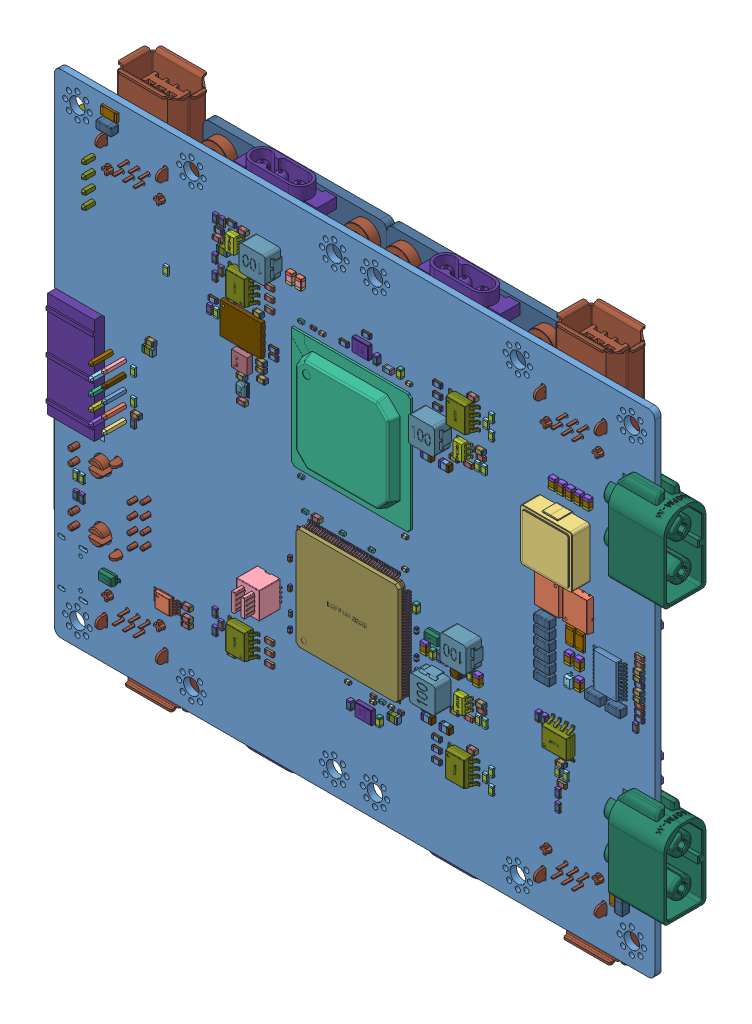
SolidWorks assembly Mother  Board, configuration 默认. Lengths in mm. (continued)
Components (placement in the parent): (continued)
- Mother  Board.step-1: Mother  Board.step [默认] at origin size (122.6 102.08 21) (continued)
  - Free-Models.step-1: Free-Models.step [默认] at origin size (70.87 98.07 8.62) (continued)
    - Driver_Board.step-1: Driver_Board.step [默认] at (49.5407 86.106 -6.2) x (-1 0 0) z (0 0 1) size (35.43 49.03 8.62) (continued)
      - C11-1.step-1: C11-1.step [默认] at origin size (1.6 0.8 0.8)
        - 6547515616.step-1: 6547515616.step [默认] at (27.6859 22.8599 0) x (-1 0 0) z (0 0 1) size (1.6 0.8 0.8)
          - Terminal-22.step-1: Terminal-22.step [默认] at (-0.8 -0.4 0) size (1.6 0.8 0.8)
            - Open_CASCADE_STEP_translator_6.8_47.1.1-85.step-1: Open_CASCADE_STEP_translator_6.8_47.1.1-85.step [默认] at origin size (0.3 0.8 0.8)
            - Open_CASCADE_STEP_translator_6.8_47.1.2-86.step-1: Open_CASCADE_STEP_translator_6.8_47.1.2-86.step [默认] at origin size (0.3 0.8 0.8)
          - Mid_Body-10.step-1: Mid_Body-10.step [默认] at (-0.8 -0.4 0) size (1 0.8 0.8)
            - Open_CASCADE_STEP_translator_6.8_47.2.1-87.step-1: Open_CASCADE_STEP_translator_6.8_47.2.1-87.step [默认] at origin size (1 0.8 0.8)
      - C10-1.step-1: C10-1.step [默认] at origin size (0.8 1.6 0.8)
        - 6547517776.step-1: 6547517776.step [默认] at (-3.1751 37.7191 0) x (0 1 0) z (0 0 1) size (1.6 0.8 0.8)
          - Terminal-24.step-1: Terminal-24.step [默认] at (-0.8 -0.4 0) size (1.6 0.8 0.8)
            - Open_CASCADE_STEP_translator_6.8_47.1.1-104.step-1: Open_CASCADE_STEP_translator_6.8_47.1.1-104.step [默认] at origin size (0.3 0.8 0.8)
            - Open_CASCADE_STEP_translator_6.8_47.1.2-105.step-1: Open_CASCADE_STEP_translator_6.8_47.1.2-105.step [默认] at origin size (0.3 0.8 0.8)
          - Mid_Body-12.step-1: Mid_Body-12.step [默认] at (-0.8 -0.4 0) size (1 0.8 0.8)
            - Open_CASCADE_STEP_translator_6.8_47.2.1-106.step-1: Open_CASCADE_STEP_translator_6.8_47.2.1-106.step [默认] at origin size (1 0.8 0.8)
      - C9-1.step-1: C9-1.step [默认] at origin size (0.8 1.6 0.8)
        - 6547516096.step-1: 6547516096.step [默认] at (-3.1749 22.2249 0) x (0 -1 0) z (0 0 1) size (1.6 0.8 0.8)
          - Terminal-23.step-1: Terminal-23.step [默认] at (-0.8 -0.4 0) size (1.6 0.8 0.8)
            - Open_CASCADE_STEP_translator_6.8_47.1.1-98.step-1: Open_CASCADE_STEP_translator_6.8_47.1.1-98.step [默认] at origin size (0.3 0.8 0.8)
            - Open_CASCADE_STEP_translator_6.8_47.1.2-99.step-1: Open_CASCADE_STEP_translator_6.8_47.1.2-99.step [默认] at origin size (0.3 0.8 0.8)
          - Mid_Body-11.step-1: Mid_Body-11.step [默认] at (-0.8 -0.4 0) size (1 0.8 0.8)
            - Open_CASCADE_STEP_translator_6.8_47.2.1-100.step-1: Open_CASCADE_STEP_translator_6.8_47.2.1-100.step [默认] at origin size (1 0.8 0.8)
      - C8-1.step-1: C8-1.step [默认] at origin size (1.6 0.8 0.8)
        - 6547515616.step-1: 6547515616.step [默认] at (1.1429 16.5099 0) x (-1 0 0) z (0 0 1) size (1.6 0.8 0.8)
          - Terminal-22.step-1: Terminal-22.step [默认] at (-0.8 -0.4 0) size (1.6 0.8 0.8)
            - Open_CASCADE_STEP_translator_6.8_47.1.1-85.step-1: Open_CASCADE_STEP_translator_6.8_47.1.1-85.step [默认] at origin size (0.3 0.8 0.8)
            - Open_CASCADE_STEP_translator_6.8_47.1.2-86.step-1: Open_CASCADE_STEP_translator_6.8_47.1.2-86.step [默认] at origin size (0.3 0.8 0.8)
          - Mid_Body-10.step-1: Mid_Body-10.step [默认] at (-0.8 -0.4 0) size (1 0.8 0.8)
            - Open_CASCADE_STEP_translator_6.8_47.2.1-87.step-1: Open_CASCADE_STEP_translator_6.8_47.2.1-87.step [默认] at origin size (1 0.8 0.8)
      - C7-1.step-1: C7-1.step [默认] at origin size (0.8 1.6 0.8)
        - 6547516096.step-1: 6547516096.step [默认] at (-2.0319 22.2249 0) x (0 -1 0) z (0 0 1) size (1.6 0.8 0.8)
          - Terminal-23.step-1: Terminal-23.step [默认] at (-0.8 -0.4 0) size (1.6 0.8 0.8)
            - Open_CASCADE_STEP_translator_6.8_47.1.1-98.step-1: Open_CASCADE_STEP_translator_6.8_47.1.1-98.step [默认] at origin size (0.3 0.8 0.8)
            - Open_CASCADE_STEP_translator_6.8_47.1.2-99.step-1: Open_CASCADE_STEP_translator_6.8_47.1.2-99.step [默认] at origin size (0.3 0.8 0.8)
          - Mid_Body-11.step-1: Mid_Body-11.step [默认] at (-0.8 -0.4 0) size (1 0.8 0.8)
            - Open_CASCADE_STEP_translator_6.8_47.2.1-100.step-1: Open_CASCADE_STEP_translator_6.8_47.2.1-100.step [默认] at origin size (1 0.8 0.8)
      - C6-1.step-1: C6-1.step [默认] at origin size (0.8 1.6 0.8)
        - 6547517776.step-1: 6547517776.step [默认] at (-2.0321 37.7191 0) x (0 1 0) z (0 0 1) size (1.6 0.8 0.8)
          - Terminal-24.step-1: Terminal-24.step [默认] at (-0.8 -0.4 0) size (1.6 0.8 0.8)
            - Open_CASCADE_STEP_translator_6.8_47.1.1-104.step-1: Open_CASCADE_STEP_translator_6.8_47.1.1-104.step [默认] at origin size (0.3 0.8 0.8)
            - Open_CASCADE_STEP_translator_6.8_47.1.2-105.step-1: Open_CASCADE_STEP_translator_6.8_47.1.2-105.step [默认] at origin size (0.3 0.8 0.8)
          - Mid_Body-12.step-1: Mid_Body-12.step [默认] at (-0.8 -0.4 0) size (1 0.8 0.8)
            - Open_CASCADE_STEP_translator_6.8_47.2.1-106.step-1: Open_CASCADE_STEP_translator_6.8_47.2.1-106.step [默认] at origin size (1 0.8 0.8)
      - C5-1.step-1: C5-1.step [默认] at origin size (1.6 0.8 0.8)
        - 6547515616.step-1: 6547515616.step [默认] at (2.7939 10.6679 0) x (-1 0 0) z (0 0 1) size (1.6 0.8 0.8)
          - Terminal-22.step-1: Terminal-22.step [默认] at (-0.8 -0.4 0) size (1.6 0.8 0.8)
            - Open_CASCADE_STEP_translator_6.8_47.1.1-85.step-1: Open_CASCADE_STEP_translator_6.8_47.1.1-85.step [默认] at origin size (0.3 0.8 0.8)
            - Open_CASCADE_STEP_translator_6.8_47.1.2-86.step-1: Open_CASCADE_STEP_translator_6.8_47.1.2-86.step [默认] at origin size (0.3 0.8 0.8)
          - Mid_Body-10.step-1: Mid_Body-10.step [默认] at (-0.8 -0.4 0) size (1 0.8 0.8)
            - Open_CASCADE_STEP_translator_6.8_47.2.1-87.step-1: Open_CASCADE_STEP_translator_6.8_47.2.1-87.step [默认] at origin size (1 0.8 0.8)
      - C4-1.step-1: C4-1.step [默认] at origin size (1.6 0.8 0.8)
        - 6547515616.step-1: 6547515616.step [默认] at (-0.1271 22.8599 0) x (-1 0 0) z (0 0 1) size (1.6 0.8 0.8)
          - Terminal-22.step-1: Terminal-22.step [默认] at (-0.8 -0.4 0) size (1.6 0.8 0.8)
            - Open_CASCADE_STEP_translator_6.8_47.1.1-85.step-1: Open_CASCADE_STEP_translator_6.8_47.1.1-85.step [默认] at origin size (0.3 0.8 0.8)
            - Open_CASCADE_STEP_translator_6.8_47.1.2-86.step-1: Open_CASCADE_STEP_translator_6.8_47.1.2-86.step [默认] at origin size (0.3 0.8 0.8)
          - Mid_Body-10.step-1: Mid_Body-10.step [默认] at (-0.8 -0.4 0) size (1 0.8 0.8)
            - Open_CASCADE_STEP_translator_6.8_47.2.1-87.step-1: Open_CASCADE_STEP_translator_6.8_47.2.1-87.step [默认] at origin size (1 0.8 0.8)
      - C3-1.step-1: C3-1.step [默认] at origin size (2.01 1.25 0.94)
        - 6547513136.step-1: 6547513136.step [默认] at (6.6263 23.4725 0) x (-1 0 0) z (0 0 1) size (2.01 1.25 0.94)
          - Fillet1-95.step-1: Fillet1-95.step [默认] at origin size (0.5 1.25 0.94)
          - Fillet2-96.step-1: Fillet2-96.step [默认] at origin size (0.5 1.25 0.94)
          - body2-97.step-1: body2-97.step [默认] at origin size (1.01 1.22 0.92)
      - C2-1.step-1: C2-1.step [默认] at origin size (0.8 1.6 0.8)
        - 6547516096.step-1: 6547516096.step [默认] at (3.7055 24.7425 0) x (0 -1 0) z (0 0 1) size (1.6 0.8 0.8)
          - Terminal-23.step-1: Terminal-23.step [默认] at (-0.8 -0.4 0) size (1.6 0.8 0.8)
            - Open_CASCADE_STEP_translator_6.8_47.1.1-98.step-1: Open_CASCADE_STEP_translator_6.8_47.1.1-98.step [默认] at origin size (0.3 0.8 0.8)
            - Open_CASCADE_STEP_translator_6.8_47.1.2-99.step-1: Open_CASCADE_STEP_translator_6.8_47.1.2-99.step [默认] at origin size (0.3 0.8 0.8)
          - Mid_Body-11.step-1: Mid_Body-11.step [默认] at (-0.8 -0.4 0) size (1 0.8 0.8)
            - Open_CASCADE_STEP_translator_6.8_47.2.1-100.step-1: Open_CASCADE_STEP_translator_6.8_47.2.1-100.step [默认] at origin size (1 0.8 0.8)
      - C1.step-1: C1.step [默认] at origin size (1.25 2.01 0.94)
        - 6547514896.step-1: 6547514896.step [默认] at (9.2933 31.0126 0) x (0 1 0) z (0 0 1) size (2.01 1.25 0.94)
          - Fillet1-101.step-1: Fillet1-101.step [默认] at origin size (0.5 1.25 0.94)
          - Fillet2-102.step-1: Fillet2-102.step [默认] at origin size (0.5 1.25 0.94)
          - body2-103.step-1: body2-103.step [默认] at origin size (1.01 1.22 0.92)
    - Driver_Board.step-2: Driver_Board.step [默认] at (84.963 86.106 -6.2) x (-1 0 0) z (0 0 1) size (35.43 49.03 8.62)
      - Board-1.step-1: Board-1.step [默认] at origin size (35.43 46.99 1.62)
        - Open_CASCADE_STEP_translator_6.8_2.1.1.step-1: Open_CASCADE_STEP_translator_6.8_2.1.1.step [默认] at (0 0 -1.6164) size (35.43 46.99 1.62)
      - R25-1.step-1: R25-1.step [默认] at origin size (0.8 1.6 0.45)
        - 6547515376.step-1: 6547515376.step [默认] at (20.6304 35.5601 0) x (0 1 0) z (0 0 1) size (1.6 0.8 0.45)
          - Terminal-19.step-1: Terminal-19.step [默认] at (-0.8 -0.4 0) size (0.3 0.8 0.45)
            - Open_CASCADE_STEP_translator_6.8_21.2.1-76.step-1: Open_CASCADE_STEP_translator_6.8_21.2.1-76.step [默认] at origin size (0.3 0.8 0.45)
          - Terminal-19.step-2: Terminal-19.step [默认] at (0.8 0.4 0) x (-1 0 0) z (0 0 1) size (0.3 0.8 0.45)
            - Open_CASCADE_STEP_translator_6.8_21.2.1-76.step-1: Open_CASCADE_STEP_translator_6.8_21.2.1-76.step [默认] at origin size (0.3 0.8 0.45)
          - Mid_Body-77.step-1: Mid_Body-77.step [默认] at (-0.8 -0.4 0) size (1.51 0.8 0.36)
          - Mark-78.step-1: Mark-78.step [默认] at (-0.5 -0.4 0.405) size (1 0.8 0.05)
      - R24-1.step-1: R24-1.step [默认] at origin size (1.6 0.8 0.45)
        - 6547516336.step-1: 6547516336.step [默认] at (12.6999 34.9249 0) x (-1 0 0) z (0 0 1) size (1.6 0.8 0.45)
          - Terminal-20.step-1: Terminal-20.step [默认] at (-0.8 -0.4 0) size (0.3 0.8 0.45)
            - Open_CASCADE_STEP_translator_6.8_21.2.1-79.step-1: Open_CASCADE_STEP_translator_6.8_21.2.1-79.step [默认] at origin size (0.3 0.8 0.45)
          - Terminal-20.step-2: Terminal-20.step [默认] at (0.8 0.4 0) x (-1 0 0) z (0 0 1) size (0.3 0.8 0.45)
            - Open_CASCADE_STEP_translator_6.8_21.2.1-79.step-1: Open_CASCADE_STEP_translator_6.8_21.2.1-79.step [默认] at origin size (0.3 0.8 0.45)
          - Mid_Body-80.step-1: Mid_Body-80.step [默认] at (-0.8 -0.4 0) size (1.51 0.8 0.36)
          - Mark-81.step-1: Mark-81.step [默认] at (-0.5 -0.4 0.405) size (1 0.8 0.05)
      - R23-1.step-1: R23-1.step [默认] at origin size (1.6 0.8 0.45)
        - 6547516336.step-1: 6547516336.step [默认] at (5.5879 33.6549 0) x (-1 0 0) z (0 0 1) size (1.6 0.8 0.45)
          - Terminal-20.step-1: Terminal-20.step [默认] at (-0.8 -0.4 0) size (0.3 0.8 0.45)
            - Open_CASCADE_STEP_translator_6.8_21.2.1-79.step-1: Open_CASCADE_STEP_translator_6.8_21.2.1-79.step [默认] at origin size (0.3 0.8 0.45)
          - Terminal-20.step-2: Terminal-20.step [默认] at (0.8 0.4 0) x (-1 0 0) z (0 0 1) size (0.3 0.8 0.45)
            - Open_CASCADE_STEP_translator_6.8_21.2.1-79.step-1: Open_CASCADE_STEP_translator_6.8_21.2.1-79.step [默认] at origin size (0.3 0.8 0.45)
          - Mid_Body-80.step-1: Mid_Body-80.step [默认] at (-0.8 -0.4 0) size (1.51 0.8 0.36)
          - Mark-81.step-1: Mark-81.step [默认] at (-0.5 -0.4 0.405) size (1 0.8 0.05)
      - JP1.step-1: JP1.step [默认] at origin size (16.01 14.49 6.96)
        - User_Library-MR30PW-M.step-1: User_Library-MR30PW-M.step [默认] at (13.7158 -5.9802 2.75) x (1 0 0) z (0 0 1) size (16.01 14.49 6.96)
      - R18-1.step-1: R18-1.step [默认] at origin size (0.8 1.6 0.45)
        - 6547515376.step-1: 6547515376.step [默认] at (22.9869 34.4171 0) x (0 1 0) z (0 0 1) size (1.6 0.8 0.45)
          - Terminal-19.step-1: Terminal-19.step [默认] at (-0.8 -0.4 0) size (0.3 0.8 0.45)
            - Open_CASCADE_STEP_translator_6.8_21.2.1-76.step-1: Open_CASCADE_STEP_translator_6.8_21.2.1-76.step [默认] at origin size (0.3 0.8 0.45)
          - Terminal-19.step-2: Terminal-19.step [默认] at (0.8 0.4 0) x (-1 0 0) z (0 0 1) size (0.3 0.8 0.45)
            - Open_CASCADE_STEP_translator_6.8_21.2.1-76.step-1: Open_CASCADE_STEP_translator_6.8_21.2.1-76.step [默认] at origin size (0.3 0.8 0.45)
          - Mid_Body-77.step-1: Mid_Body-77.step [默认] at (-0.8 -0.4 0) size (1.51 0.8 0.36)
          - Mark-78.step-1: Mark-78.step [默认] at (-0.5 -0.4 0.405) size (1 0.8 0.05)
      - R17-1.step-1: R17-1.step [默认] at origin size (0.8 1.6 0.45)
        - 6547515376.step-1: 6547515376.step [默认] at (21.8663 34.3947 0) x (0 1 0) z (0 0 1) size (1.6 0.8 0.45)
          - Terminal-19.step-1: Terminal-19.step [默认] at (-0.8 -0.4 0) size (0.3 0.8 0.45)
            - Open_CASCADE_STEP_translator_6.8_21.2.1-76.step-1: Open_CASCADE_STEP_translator_6.8_21.2.1-76.step [默认] at origin size (0.3 0.8 0.45)
          - Terminal-19.step-2: Terminal-19.step [默认] at (0.8 0.4 0) x (-1 0 0) z (0 0 1) size (0.3 0.8 0.45)
            - Open_CASCADE_STEP_translator_6.8_21.2.1-76.step-1: Open_CASCADE_STEP_translator_6.8_21.2.1-76.step [默认] at origin size (0.3 0.8 0.45)
          - Mid_Body-77.step-1: Mid_Body-77.step [默认] at (-0.8 -0.4 0) size (1.51 0.8 0.36)
          - Mark-78.step-1: Mark-78.step [默认] at (-0.5 -0.4 0.405) size (1 0.8 0.05)
      - R16-1.step-1: R16-1.step [默认] at origin size (1.6 0.8 0.45)
        - 6547506496.step-1: 6547506496.step [默认] at (16.6371 33.6551 0) x (1 0 0) z (0 0 1) size (1.6 0.8 0.45)
          - Terminal-21.step-1: Terminal-21.step [默认] at (-0.8 -0.4 0) size (0.3 0.8 0.45)
            - Open_CASCADE_STEP_translator_6.8_21.2.1-82.step-1: Open_CASCADE_STEP_translator_6.8_21.2.1-82.step [默认] at origin size (0.3 0.8 0.45)
          - Terminal-21.step-2: Terminal-21.step [默认] at (0.8 0.4 0) x (-1 0 0) z (0 0 1) size (0.3 0.8 0.45)
            - Open_CASCADE_STEP_translator_6.8_21.2.1-82.step-1: Open_CASCADE_STEP_translator_6.8_21.2.1-82.step [默认] at origin size (0.3 0.8 0.45)
          - Mid_Body-83.step-1: Mid_Body-83.step [默认] at (-0.8 -0.4 0) size (1.51 0.8 0.36)
          - Mark-84.step-1: Mark-84.step [默认] at (-0.5 -0.4 0.405) size (1 0.8 0.05)
      - R15-1.step-1: R15-1.step [默认] at origin size (0.8 1.6 0.45)
        - 6547515376.step-1: 6547515376.step [默认] at (14.7319 34.2901 0) x (0 1 0) z (0 0 1) size (1.6 0.8 0.45)
          - Terminal-19.step-1: Terminal-19.step [默认] at (-0.8 -0.4 0) size (0.3 0.8 0.45)
            - Open_CASCADE_STEP_translator_6.8_21.2.1-76.step-1: Open_CASCADE_STEP_translator_6.8_21.2.1-76.step [默认] at origin size (0.3 0.8 0.45)
          - Terminal-19.step-2: Terminal-19.step [默认] at (0.8 0.4 0) x (-1 0 0) z (0 0 1) size (0.3 0.8 0.45)
            - Open_CASCADE_STEP_translator_6.8_21.2.1-76.step-1: Open_CASCADE_STEP_translator_6.8_21.2.1-76.step [默认] at origin size (0.3 0.8 0.45)
          - Mid_Body-77.step-1: Mid_Body-77.step [默认] at (-0.8 -0.4 0) size (1.51 0.8 0.36)
          - Mark-78.step-1: Mark-78.step [默认] at (-0.5 -0.4 0.405) size (1 0.8 0.05)
      - R13-1.step-1: R13-1.step [默认] at origin size (1.6 0.8 0.45)
        - 6547506496.step-1: 6547506496.step [默认] at (9.5251 33.6551 0) x (1 0 0) z (0 0 1) size (1.6 0.8 0.45)
          - Terminal-21.step-1: Terminal-21.step [默认] at (-0.8 -0.4 0) size (0.3 0.8 0.45)
            - Open_CASCADE_STEP_translator_6.8_21.2.1-82.step-1: Open_CASCADE_STEP_translator_6.8_21.2.1-82.step [默认] at origin size (0.3 0.8 0.45)
          - Terminal-21.step-2: Terminal-21.step [默认] at (0.8 0.4 0) x (-1 0 0) z (0 0 1) size (0.3 0.8 0.45)
            - Open_CASCADE_STEP_translator_6.8_21.2.1-82.step-1: Open_CASCADE_STEP_translator_6.8_21.2.1-82.step [默认] at origin size (0.3 0.8 0.45)
          - Mid_Body-83.step-1: Mid_Body-83.step [默认] at (-0.8 -0.4 0) size (1.51 0.8 0.36)
          - Mark-84.step-1: Mark-84.step [默认] at (-0.5 -0.4 0.405) size (1 0.8 0.05)
      - R11-1.step-1: R11-1.step [默认] at origin size (0.8 1.6 0.45)
        - 6547515376.step-1: 6547515376.step [默认] at (7.6423 34.2901 0) x (0 1 0) z (0 0 1) size (1.6 0.8 0.45)
          - Terminal-19.step-1: Terminal-19.step [默认] at (-0.8 -0.4 0) size (0.3 0.8 0.45)
            - Open_CASCADE_STEP_translator_6.8_21.2.1-76.step-1: Open_CASCADE_STEP_translator_6.8_21.2.1-76.step [默认] at origin size (0.3 0.8 0.45)
          - Terminal-19.step-2: Terminal-19.step [默认] at (0.8 0.4 0) x (-1 0 0) z (0 0 1) size (0.3 0.8 0.45)
            - Open_CASCADE_STEP_translator_6.8_21.2.1-76.step-1: Open_CASCADE_STEP_translator_6.8_21.2.1-76.step [默认] at origin size (0.3 0.8 0.45)
          - Mid_Body-77.step-1: Mid_Body-77.step [默认] at (-0.8 -0.4 0) size (1.51 0.8 0.36)
          - Mark-78.step-1: Mark-78.step [默认] at (-0.5 -0.4 0.405) size (1 0.8 0.05)
      - C23-1.step-1: C23-1.step [默认] at origin size (1.6 0.8 0.8)
        - 6547515616.step-1: 6547515616.step [默认] at (19.8684 33.6676 0) x (-1 0 0) z (0 0 1) size (1.6 0.8 0.8)
          - Terminal-22.step-1: Terminal-22.step [默认] at (-0.8 -0.4 0) size (1.6 0.8 0.8)
            - Open_CASCADE_STEP_translator_6.8_47.1.1-85.step-1: Open_CASCADE_STEP_translator_6.8_47.1.1-85.step [默认] at origin size (0.3 0.8 0.8)
            - Open_CASCADE_STEP_translator_6.8_47.1.2-86.step-1: Open_CASCADE_STEP_translator_6.8_47.1.2-86.step [默认] at origin size (0.3 0.8 0.8)
          - Mid_Body-10.step-1: Mid_Body-10.step [默认] at (-0.8 -0.4 0) size (1 0.8 0.8)
            - Open_CASCADE_STEP_translator_6.8_47.2.1-87.step-1: Open_CASCADE_STEP_translator_6.8_47.2.1-87.step [默认] at origin size (1 0.8 0.8)
      - C22-1.step-1: C22-1.step [默认] at origin size (1.6 0.8 0.8)
        - 6547515616.step-1: 6547515616.step [默认] at (12.6999 33.6549 0) x (-1 0 0) z (0 0 1) size (1.6 0.8 0.8)
          - Terminal-22.step-1: Terminal-22.step [默认] at (-0.8 -0.4 0) size (1.6 0.8 0.8)
            - Open_CASCADE_STEP_translator_6.8_47.1.1-85.step-1: Open_CASCADE_STEP_translator_6.8_47.1.1-85.step [默认] at origin size (0.3 0.8 0.8)
            - Open_CASCADE_STEP_translator_6.8_47.1.2-86.step-1: Open_CASCADE_STEP_translator_6.8_47.1.2-86.step [默认] at origin size (0.3 0.8 0.8)
          - Mid_Body-10.step-1: Mid_Body-10.step [默认] at (-0.8 -0.4 0) size (1 0.8 0.8)
            - Open_CASCADE_STEP_translator_6.8_47.2.1-87.step-1: Open_CASCADE_STEP_translator_6.8_47.2.1-87.step [默认] at origin size (1 0.8 0.8)
      - C21-1.step-1: C21-1.step [默认] at origin size (1.6 0.8 0.8)
        - 6547515616.step-1: 6547515616.step [默认] at (5.6103 34.9025 0) x (-1 0 0) z (0 0 1) size (1.6 0.8 0.8)
          - Terminal-22.step-1: Terminal-22.step [默认] at (-0.8 -0.4 0) size (1.6 0.8 0.8)
            - Open_CASCADE_STEP_translator_6.8_47.1.1-85.step-1: Open_CASCADE_STEP_translator_6.8_47.1.1-85.step [默认] at origin size (0.3 0.8 0.8)
            - Open_CASCADE_STEP_translator_6.8_47.1.2-86.step-1: Open_CASCADE_STEP_translator_6.8_47.1.2-86.step [默认] at origin size (0.3 0.8 0.8)
          - Mid_Body-10.step-1: Mid_Body-10.step [默认] at (-0.8 -0.4 0) size (1 0.8 0.8)
            - Open_CASCADE_STEP_translator_6.8_47.2.1-87.step-1: Open_CASCADE_STEP_translator_6.8_47.2.1-87.step [默认] at origin size (1 0.8 0.8)
      - U5-1.step-1: U5-1.step [默认] at origin size (5.9 11.5 2.7)
        - SO8_W.step-1: SO8_W.step [默认] at (27.6859 29.9721 0.381) x (0 1 0) z (0 0 1) size (11.5 5.9 2.7)
      - U4-1.step-1: U4-1.step [默认] at origin size (5.9 11.5 2.7)
        - SO8_W.step-1: SO8_W.step [默认] at (-0.1271 29.9721 0.381) x (0 1 0) z (0 0 1) size (11.5 5.9 2.7)
      - U3-1.step-1: U3-1.step [默认] at origin size (5 6.01 1.9)
        - SOP8-1.step-1: SOP8-1.step [默认] at (19.9615 29.5285 0) x (0 -1 0) z (0 0 1) size (6.01 5 1.9)
          - LOGO_-88.step-1: LOGO_-88.step [默认] at (0.0116 0 0.095) x (0 -1 0) z (0 0 -1) size (1.5 1.73 0.01)
          - SOP8-89.step-1: SOP8-89.step [默认] at origin size (6.01 5 1.9)
      - U2-1.step-1: U2-1.step [默认] at origin size (5 6.01 1.9)
        - SOP8-1.step-1: SOP8-1.step [默认] at (12.8495 29.5285 0) x (0 -1 0) z (0 0 1) size (6.01 5 1.9)
          - LOGO_-88.step-1: LOGO_-88.step [默认] at (0.0116 0 0.095) x (0 -1 0) z (0 0 -1) size (1.5 1.73 0.01)
          - SOP8-89.step-1: SOP8-89.step [默认] at origin size (6.01 5 1.9)
      - U1.step-1: U1.step [默认] at origin size (5 6.01 1.9)
        - SOP8-1.step-1: SOP8-1.step [默认] at (5.7375 29.5285 0) x (0 -1 0) z (0 0 1) size (6.01 5 1.9)
          - LOGO_-88.step-1: LOGO_-88.step [默认] at (0.0116 0 0.095) x (0 -1 0) z (0 0 -1) size (1.5 1.73 0.01)
          - SOP8-89.step-1: SOP8-89.step [默认] at origin size (6.01 5 1.9)
      - RS2-1.step-1: RS2-1.step [默认] at origin size (3.1 1.55 0.47)
        - User_Library-R1206-90.step-1: User_Library-R1206-90.step [默认] at (23.7489 17.5261 -1.6164) x (-1 0 0) z (0 0 -1) size (3.1 1.55 0.47)
      - RS1-1.step-1: RS1-1.step [默认] at origin size (3.1 1.55 0.47)
        - User_Library-R1206-90.step-1: User_Library-R1206-90.step [默认] at (-0.1271 18.1611 -1.6164) x (-1 0 0) z (0 0 -1) size (3.1 1.55 0.47)
      - R22-1.step-1: R22-1.step [默认] at origin size (1.6 0.8 0.45)
        - 6547506496.step-1: 6547506496.step [默认] at (22.9871 17.7801 0) x (1 0 0) z (0 0 1) size (1.6 0.8 0.45)
          - Terminal-21.step-1: Terminal-21.step [默认] at (-0.8 -0.4 0) size (0.3 0.8 0.45)
            - Open_CASCADE_STEP_translator_6.8_21.2.1-82.step-1: Open_CASCADE_STEP_translator_6.8_21.2.1-82.step [默认] at origin size (0.3 0.8 0.45)
          - Terminal-21.step-2: Terminal-21.step [默认] at (0.8 0.4 0) x (-1 0 0) z (0 0 1) size (0.3 0.8 0.45)
            - Open_CASCADE_STEP_translator_6.8_21.2.1-82.step-1: Open_CASCADE_STEP_translator_6.8_21.2.1-82.step [默认] at origin size (0.3 0.8 0.45)
          - Mid_Body-83.step-1: Mid_Body-83.step [默认] at (-0.8 -0.4 0) size (1.51 0.8 0.36)
          - Mark-84.step-1: Mark-84.step [默认] at (-0.5 -0.4 0.405) size (1 0.8 0.05)
      - R21-1.step-1: R21-1.step [默认] at origin size (1.6 0.8 0.45)
        - 6547516336.step-1: 6547516336.step [默认] at (22.9869 18.9229 0) x (-1 0 0) z (0 0 1) size (1.6 0.8 0.45)
          - Terminal-20.step-1: Terminal-20.step [默认] at (-0.8 -0.4 0) size (0.3 0.8 0.45)
            - Open_CASCADE_STEP_translator_6.8_21.2.1-79.step-1: Open_CASCADE_STEP_translator_6.8_21.2.1-79.step [默认] at origin size (0.3 0.8 0.45)
          - Terminal-20.step-2: Terminal-20.step [默认] at (0.8 0.4 0) x (-1 0 0) z (0 0 1) size (0.3 0.8 0.45)
            - Open_CASCADE_STEP_translator_6.8_21.2.1-79.step-1: Open_CASCADE_STEP_translator_6.8_21.2.1-79.step [默认] at origin size (0.3 0.8 0.45)
          - Mid_Body-80.step-1: Mid_Body-80.step [默认] at (-0.8 -0.4 0) size (1.51 0.8 0.36)
          - Mark-81.step-1: Mark-81.step [默认] at (-0.5 -0.4 0.405) size (1 0.8 0.05)
      - R20-1.step-1: R20-1.step [默认] at origin size (1.6 0.8 0.45)
        - 6547506496.step-1: 6547506496.step [默认] at (24.6381 11.8111 0) x (1 0 0) z (0 0 1) size (1.6 0.8 0.45)
          - Terminal-21.step-1: Terminal-21.step [默认] at (-0.8 -0.4 0) size (0.3 0.8 0.45)
            - Open_CASCADE_STEP_translator_6.8_21.2.1-82.step-1: Open_CASCADE_STEP_translator_6.8_21.2.1-82.step [默认] at origin size (0.3 0.8 0.45)
          - Terminal-21.step-2: Terminal-21.step [默认] at (0.8 0.4 0) x (-1 0 0) z (0 0 1) size (0.3 0.8 0.45)
            - Open_CASCADE_STEP_translator_6.8_21.2.1-82.step-1: Open_CASCADE_STEP_translator_6.8_21.2.1-82.step [默认] at origin size (0.3 0.8 0.45)
          - Mid_Body-83.step-1: Mid_Body-83.step [默认] at (-0.8 -0.4 0) size (1.51 0.8 0.36)
          - Mark-84.step-1: Mark-84.step [默认] at (-0.5 -0.4 0.405) size (1 0.8 0.05)
      - R19-1.step-1: R19-1.step [默认] at origin size (0.8 1.6 0.45)
        - 6547515376.step-1: 6547515376.step [默认] at (25.3999 13.5891 0) x (0 1 0) z (0 0 1) size (1.6 0.8 0.45)
          - Terminal-19.step-1: Terminal-19.step [默认] at (-0.8 -0.4 0) size (0.3 0.8 0.45)
            - Open_CASCADE_STEP_translator_6.8_21.2.1-76.step-1: Open_CASCADE_STEP_translator_6.8_21.2.1-76.step [默认] at origin size (0.3 0.8 0.45)
          - Terminal-19.step-2: Terminal-19.step [默认] at (0.8 0.4 0) x (-1 0 0) z (0 0 1) size (0.3 0.8 0.45)
            - Open_CASCADE_STEP_translator_6.8_21.2.1-76.step-1: Open_CASCADE_STEP_translator_6.8_21.2.1-76.step [默认] at origin size (0.3 0.8 0.45)
          - Mid_Body-77.step-1: Mid_Body-77.step [默认] at (-0.8 -0.4 0) size (1.51 0.8 0.36)
          - Mark-78.step-1: Mark-78.step [默认] at (-0.5 -0.4 0.405) size (1 0.8 0.05)
      - R14-1.step-1: R14-1.step [默认] at origin size (1.6 0.8 0.45)
        - 6547506496.step-1: 6547506496.step [默认] at (12.0651 20.0661 0) x (1 0 0) z (0 0 1) size (1.6 0.8 0.45)
          - Terminal-21.step-1: Terminal-21.step [默认] at (-0.8 -0.4 0) size (0.3 0.8 0.45)
            - Open_CASCADE_STEP_translator_6.8_21.2.1-82.step-1: Open_CASCADE_STEP_translator_6.8_21.2.1-82.step [默认] at origin size (0.3 0.8 0.45)
          - Terminal-21.step-2: Terminal-21.step [默认] at (0.8 0.4 0) x (-1 0 0) z (0 0 1) size (0.3 0.8 0.45)
            - Open_CASCADE_STEP_translator_6.8_21.2.1-82.step-1: Open_CASCADE_STEP_translator_6.8_21.2.1-82.step [默认] at origin size (0.3 0.8 0.45)
          - Mid_Body-83.step-1: Mid_Body-83.step [默认] at (-0.8 -0.4 0) size (1.51 0.8 0.36)
          - Mark-84.step-1: Mark-84.step [默认] at (-0.5 -0.4 0.405) size (1 0.8 0.05)
      - R12-1.step-1: R12-1.step [默认] at origin size (1.6 0.8 0.45)
        - 6547516336.step-1: 6547516336.step [默认] at (12.0649 21.2089 0) x (-1 0 0) z (0 0 1) size (1.6 0.8 0.45)
          - Terminal-20.step-1: Terminal-20.step [默认] at (-0.8 -0.4 0) size (0.3 0.8 0.45)
            - Open_CASCADE_STEP_translator_6.8_21.2.1-79.step-1: Open_CASCADE_STEP_translator_6.8_21.2.1-79.step [默认] at origin size (0.3 0.8 0.45)
          - Terminal-20.step-2: Terminal-20.step [默认] at (0.8 0.4 0) x (-1 0 0) z (0 0 1) size (0.3 0.8 0.45)
            - Open_CASCADE_STEP_translator_6.8_21.2.1-79.step-1: Open_CASCADE_STEP_translator_6.8_21.2.1-79.step [默认] at origin size (0.3 0.8 0.45)
          - Mid_Body-80.step-1: Mid_Body-80.step [默认] at (-0.8 -0.4 0) size (1.51 0.8 0.36)
          - Mark-81.step-1: Mark-81.step [默认] at (-0.5 -0.4 0.405) size (1 0.8 0.05)
      - R10-1.step-1: R10-1.step [默认] at origin size (1.6 0.8 0.45)
        - 6547506496.step-1: 6547506496.step [默认] at (13.7161 14.0971 0) x (1 0 0) z (0 0 1) size (1.6 0.8 0.45)
          - Terminal-21.step-1: Terminal-21.step [默认] at (-0.8 -0.4 0) size (0.3 0.8 0.45)
            - Open_CASCADE_STEP_translator_6.8_21.2.1-82.step-1: Open_CASCADE_STEP_translator_6.8_21.2.1-82.step [默认] at origin size (0.3 0.8 0.45)
          - Terminal-21.step-2: Terminal-21.step [默认] at (0.8 0.4 0) x (-1 0 0) z (0 0 1) size (0.3 0.8 0.45)
            - Open_CASCADE_STEP_translator_6.8_21.2.1-82.step-1: Open_CASCADE_STEP_translator_6.8_21.2.1-82.step [默认] at origin size (0.3 0.8 0.45)
          - Mid_Body-83.step-1: Mid_Body-83.step [默认] at (-0.8 -0.4 0) size (1.51 0.8 0.36)
          - Mark-84.step-1: Mark-84.step [默认] at (-0.5 -0.4 0.405) size (1 0.8 0.05)
      - R9-1.step-1: R9-1.step [默认] at origin size (0.8 1.6 0.45)
        - 6547515376.step-1: 6547515376.step [默认] at (14.4779 15.8751 0) x (0 1 0) z (0 0 1) size (1.6 0.8 0.45)
          - Terminal-19.step-1: Terminal-19.step [默认] at (-0.8 -0.4 0) size (0.3 0.8 0.45)
            - Open_CASCADE_STEP_translator_6.8_21.2.1-76.step-1: Open_CASCADE_STEP_translator_6.8_21.2.1-76.step [默认] at origin size (0.3 0.8 0.45)
          - Terminal-19.step-2: Terminal-19.step [默认] at (0.8 0.4 0) x (-1 0 0) z (0 0 1) size (0.3 0.8 0.45)
            - Open_CASCADE_STEP_translator_6.8_21.2.1-76.step-1: Open_CASCADE_STEP_translator_6.8_21.2.1-76.step [默认] at origin size (0.3 0.8 0.45)
          - Mid_Body-77.step-1: Mid_Body-77.step [默认] at (-0.8 -0.4 0) size (1.51 0.8 0.36)
          - Mark-78.step-1: Mark-78.step [默认] at (-0.5 -0.4 0.405) size (1 0.8 0.05)
      - R8-1.step-1: R8-1.step [默认] at origin size (0.8 1.6 0.45)
        - 6547515376.step-1: 6547515376.step [默认] at (28.3209 21.0821 0) x (0 1 0) z (0 0 1) size (1.6 0.8 0.45)
          - Terminal-19.step-1: Terminal-19.step [默认] at (-0.8 -0.4 0) size (0.3 0.8 0.45)
            - Open_CASCADE_STEP_translator_6.8_21.2.1-76.step-1: Open_CASCADE_STEP_translator_6.8_21.2.1-76.step [默认] at origin size (0.3 0.8 0.45)
          - Terminal-19.step-2: Terminal-19.step [默认] at (0.8 0.4 0) x (-1 0 0) z (0 0 1) size (0.3 0.8 0.45)
            - Open_CASCADE_STEP_translator_6.8_21.2.1-76.step-1: Open_CASCADE_STEP_translator_6.8_21.2.1-76.step [默认] at origin size (0.3 0.8 0.45)
          - Mid_Body-77.step-1: Mid_Body-77.step [默认] at (-0.8 -0.4 0) size (1.51 0.8 0.36)
          - Mark-78.step-1: Mark-78.step [默认] at (-0.5 -0.4 0.405) size (1 0.8 0.05)
      - R7-1.step-1: R7-1.step [默认] at origin size (0.8 1.6 0.45)
        - 6547515376.step-1: 6547515376.step [默认] at (27.0509 21.0821 0) x (0 1 0) z (0 0 1) size (1.6 0.8 0.45)
          - Terminal-19.step-1: Terminal-19.step [默认] at (-0.8 -0.4 0) size (0.3 0.8 0.45)
            - Open_CASCADE_STEP_translator_6.8_21.2.1-76.step-1: Open_CASCADE_STEP_translator_6.8_21.2.1-76.step [默认] at origin size (0.3 0.8 0.45)
          - Terminal-19.step-2: Terminal-19.step [默认] at (0.8 0.4 0) x (-1 0 0) z (0 0 1) size (0.3 0.8 0.45)
            - Open_CASCADE_STEP_translator_6.8_21.2.1-76.step-1: Open_CASCADE_STEP_translator_6.8_21.2.1-76.step [默认] at origin size (0.3 0.8 0.45)
          - Mid_Body-77.step-1: Mid_Body-77.step [默认] at (-0.8 -0.4 0) size (1.51 0.8 0.36)
          - Mark-78.step-1: Mark-78.step [默认] at (-0.5 -0.4 0.405) size (1 0.8 0.05)
      - R6.step-1: R6.step [默认] at origin size (1.6 0.8 0.45)
        - 6547506496.step-1: 6547506496.step [默认] at (1.1431 17.6531 0) x (1 0 0) z (0 0 1) size (1.6 0.8 0.45)
          - Terminal-21.step-1: Terminal-21.step [默认] at (-0.8 -0.4 0) size (0.3 0.8 0.45)
            - Open_CASCADE_STEP_translator_6.8_21.2.1-82.step-1: Open_CASCADE_STEP_translator_6.8_21.2.1-82.step [默认] at origin size (0.3 0.8 0.45)
          - Terminal-21.step-2: Terminal-21.step [默认] at (0.8 0.4 0) x (-1 0 0) z (0 0 1) size (0.3 0.8 0.45)
            - Open_CASCADE_STEP_translator_6.8_21.2.1-82.step-1: Open_CASCADE_STEP_translator_6.8_21.2.1-82.step [默认] at origin size (0.3 0.8 0.45)
          - Mid_Body-83.step-1: Mid_Body-83.step [默认] at (-0.8 -0.4 0) size (1.51 0.8 0.36)
          - Mark-84.step-1: Mark-84.step [默认] at (-0.5 -0.4 0.405) size (1 0.8 0.05)
      - R5.step-1: R5.step [默认] at origin size (0.8 1.6 0.45)
        - 6547515376.step-1: 6547515376.step [默认] at (1.7779 21.0821 0) x (0 1 0) z (0 0 1) size (1.6 0.8 0.45)
          - Terminal-19.step-1: Terminal-19.step [默认] at (-0.8 -0.4 0) size (0.3 0.8 0.45)
            - Open_CASCADE_STEP_translator_6.8_21.2.1-76.step-1: Open_CASCADE_STEP_translator_6.8_21.2.1-76.step [默认] at origin size (0.3 0.8 0.45)
          - Terminal-19.step-2: Terminal-19.step [默认] at (0.8 0.4 0) x (-1 0 0) z (0 0 1) size (0.3 0.8 0.45)
            - Open_CASCADE_STEP_translator_6.8_21.2.1-76.step-1: Open_CASCADE_STEP_translator_6.8_21.2.1-76.step [默认] at origin size (0.3 0.8 0.45)
          - Mid_Body-77.step-1: Mid_Body-77.step [默认] at (-0.8 -0.4 0) size (1.51 0.8 0.36)
          - Mark-78.step-1: Mark-78.step [默认] at (-0.5 -0.4 0.405) size (1 0.8 0.05)
      - R4.step-1: R4.step [默认] at origin size (0.8 1.6 0.45)
        - 6547515376.step-1: 6547515376.step [默认] at (0.5079 21.0821 0) x (0 1 0) z (0 0 1) size (1.6 0.8 0.45)
          - Terminal-19.step-1: Terminal-19.step [默认] at (-0.8 -0.4 0) size (0.3 0.8 0.45)
            - Open_CASCADE_STEP_translator_6.8_21.2.1-76.step-1: Open_CASCADE_STEP_translator_6.8_21.2.1-76.step [默认] at origin size (0.3 0.8 0.45)
          - Terminal-19.step-2: Terminal-19.step [默认] at (0.8 0.4 0) x (-1 0 0) z (0 0 1) size (0.3 0.8 0.45)
            - Open_CASCADE_STEP_translator_6.8_21.2.1-76.step-1: Open_CASCADE_STEP_translator_6.8_21.2.1-76.step [默认] at origin size (0.3 0.8 0.45)
          - Mid_Body-77.step-1: Mid_Body-77.step [默认] at (-0.8 -0.4 0) size (1.51 0.8 0.36)
          - Mark-78.step-1: Mark-78.step [默认] at (-0.5 -0.4 0.405) size (1 0.8 0.05)
      - R3.step-1: R3.step [默认] at origin size (1.6 0.8 0.45)
        - 6547506496.step-1: 6547506496.step [默认] at (2.7941 11.8111 0) x (1 0 0) z (0 0 1) size (1.6 0.8 0.45)
          - Terminal-21.step-1: Terminal-21.step [默认] at (-0.8 -0.4 0) size (0.3 0.8 0.45)
            - Open_CASCADE_STEP_translator_6.8_21.2.1-82.step-1: Open_CASCADE_STEP_translator_6.8_21.2.1-82.step [默认] at origin size (0.3 0.8 0.45)
          - Terminal-21.step-2: Terminal-21.step [默认] at (0.8 0.4 0) x (-1 0 0) z (0 0 1) size (0.3 0.8 0.45)
            - Open_CASCADE_STEP_translator_6.8_21.2.1-82.step-1: Open_CASCADE_STEP_translator_6.8_21.2.1-82.step [默认] at origin size (0.3 0.8 0.45)
          - Mid_Body-83.step-1: Mid_Body-83.step [默认] at (-0.8 -0.4 0) size (1.51 0.8 0.36)
          - Mark-84.step-1: Mark-84.step [默认] at (-0.5 -0.4 0.405) size (1 0.8 0.05)
      - R2.step-1: R2.step [默认] at origin size (0.8 1.6 0.45)
        - 6547515376.step-1: 6547515376.step [默认] at (-0.7621 21.0821 0) x (0 1 0) z (0 0 1) size (1.6 0.8 0.45)
          - Terminal-19.step-1: Terminal-19.step [默认] at (-0.8 -0.4 0) size (0.3 0.8 0.45)
            - Open_CASCADE_STEP_translator_6.8_21.2.1-76.step-1: Open_CASCADE_STEP_translator_6.8_21.2.1-76.step [默认] at origin size (0.3 0.8 0.45)
          - Terminal-19.step-2: Terminal-19.step [默认] at (0.8 0.4 0) x (-1 0 0) z (0 0 1) size (0.3 0.8 0.45)
            - Open_CASCADE_STEP_translator_6.8_21.2.1-76.step-1: Open_CASCADE_STEP_translator_6.8_21.2.1-76.step [默认] at origin size (0.3 0.8 0.45)
          - Mid_Body-77.step-1: Mid_Body-77.step [默认] at (-0.8 -0.4 0) size (1.51 0.8 0.36)
          - Mark-78.step-1: Mark-78.step [默认] at (-0.5 -0.4 0.405) size (1 0.8 0.05)
      - R1.step-1: R1.step [默认] at origin size (0.8 1.6 0.45)
        - 6547515376.step-1: 6547515376.step [默认] at (3.5559 13.5891 0) x (0 1 0) z (0 0 1) size (1.6 0.8 0.45)
          - Terminal-19.step-1: Terminal-19.step [默认] at (-0.8 -0.4 0) size (0.3 0.8 0.45)
            - Open_CASCADE_STEP_translator_6.8_21.2.1-76.step-1: Open_CASCADE_STEP_translator_6.8_21.2.1-76.step [默认] at origin size (0.3 0.8 0.45)
          - Terminal-19.step-2: Terminal-19.step [默认] at (0.8 0.4 0) x (-1 0 0) z (0 0 1) size (0.3 0.8 0.45)
            - Open_CASCADE_STEP_translator_6.8_21.2.1-76.step-1: Open_CASCADE_STEP_translator_6.8_21.2.1-76.step [默认] at origin size (0.3 0.8 0.45)
          - Mid_Body-77.step-1: Mid_Body-77.step [默认] at (-0.8 -0.4 0) size (1.51 0.8 0.36)
          - Mark-78.step-1: Mark-78.step [默认] at (-0.5 -0.4 0.405) size (1 0.8 0.05)
      - M6.step-1: M6.step [默认] at origin size (5.15 6.15 1.1)
        - TDSON-8-91.step-1: TDSON-8-91.step [默认] at (21.8441 12.7711 -1.6164) x (1 0 0) z (0 1 0) size (5.15 1.1 6.15)
      - M5.step-1: M5.step [默认] at origin size (5.15 6.15 1.1)
        - TDSON-8-91.step-1: TDSON-8-91.step [默认] at (27.3049 12.7713 -1.6164) x (-1 0 0) z (0 -1 0) size (5.15 1.1 6.15)
      - M4.step-1: M4.step [默认] at origin size (5.15 6.15 1.1)
        - TDSON-8-91.step-1: TDSON-8-91.step [默认] at (10.9221 15.0571 -1.6164) x (1 0 0) z (0 1 0) size (5.15 1.1 6.15)
      - M3.step-1: M3.step [默认] at origin size (5.15 6.15 1.1)
        - TDSON-8-91.step-1: TDSON-8-91.step [默认] at (16.3829 15.0573 -1.6164) x (-1 0 0) z (0 -1 0) size (5.15 1.1 6.15)
      - M2-1.step-1: M2-1.step [默认] at origin size (5.15 6.15 1.1)
        - TDSON-8-91.step-1: TDSON-8-91.step [默认] at (0 12.7711 -1.6164) x (1 0 0) z (0 1 0) size (5.15 1.1 6.15)
      - M1-1.step-1: M1-1.step [默认] at origin size (5.15 6.15 1.1)
        - TDSON-8-91.step-1: TDSON-8-91.step [默认] at (5.4609 12.7713 -1.6164) x (-1 0 0) z (0 -1 0) size (5.15 1.1 6.15)
      - JP4-1.step-1: JP4-1.step [默认] at origin size (5.56 5.56 4.53)
        - User_Library-SMTSO-M3-3ET.step-1: User_Library-SMTSO-M3-3ET.step [默认] at (27.5589 0.0001 -2.6164) x (0 0 1) z (0 1 0) size (4.53 5.56 5.56)
      - JP3-1.step-1: JP3-1.step [默认] at origin size (5.56 5.56 4.53)
        - User_Library-SMTSO-M3-3ET.step-1: User_Library-SMTSO-M3-3ET.step [默认] at (-0.0001 0.0001 -2.6164) x (0 0 1) z (0 1 0) size (4.53 5.56 5.56)
      - JP2.step-1: JP2.step [默认] at origin size (11.5 4.96 6.5)
        - SG340-GxxP-B1-2x12.step-1: SG340-GxxP-B1-2x12.step [默认] at (13.7793 38.9891 0) x (-1 0 0) z (0 0 1) size (11.5 4.96 6.5)
      - D3-1.step-1: D3-1.step [默认] at origin size (2.65 1.3 0.96)
        - SOD-323-1.step-1: SOD-323-1.step [默认] at (20.5836 25.1426 0.05) x (-1 0 0) z (0 0 1) size (2.65 1.3 0.96)
          - SOD-323-92.step-1: SOD-323-92.step [默认] at origin size (2.65 1.3 0.95)
          - LOGO______.__-93.step-1: LOGO______.__-93.step [默认] at (0.0033 0.0815 -0.003) x (-1 0 0) z (0 0 -1) size (0.9 1.04 0.01)
      - D2-1.step-1: D2-1.step [默认] at origin size (2.65 1.3 0.96)
        - SOD-323-1.step-1: SOD-323-1.step [默认] at (13.4716 25.1426 0.05) x (-1 0 0) z (0 0 1) size (2.65 1.3 0.96)
          - SOD-323-92.step-1: SOD-323-92.step [默认] at origin size (2.65 1.3 0.95)
          - LOGO______.__-93.step-1: LOGO______.__-93.step [默认] at (0.0033 0.0815 -0.003) x (-1 0 0) z (0 0 -1) size (0.9 1.04 0.01)
      - D1-1.step-1: D1-1.step [默认] at origin size (2.65 1.3 0.96)
        - SOD-323-1.step-1: SOD-323-1.step [默认] at (6.3596 25.1426 0.05) x (-1 0 0) z (0 0 1) size (2.65 1.3 0.96)
          - SOD-323-92.step-1: SOD-323-92.step [默认] at origin size (2.65 1.3 0.95)
          - LOGO______.__-93.step-1: LOGO______.__-93.step [默认] at (0.0033 0.0815 -0.003) x (-1 0 0) z (0 0 -1) size (0.9 1.04 0.01)
      - CP7-1.step-1: CP7-1.step [默认] at origin size (1.5 3 1.5)
        - (______)-94.step-1: (______)-94.step [默认] at (29.2101 17.1449 0) x (1 0 0) z (0 0 1) size (1.5 3 1.5)
      - CP9.step-1: CP9.step [默认] at origin size (1.5 3 1.5)
        - (______)-94.step-1: (______)-94.step [默认] at (18.2881 19.4309 0) x (1 0 0) z (0 0 1) size (1.5 3 1.5)
      - CP8-1.step-1: CP8-1.step [默认] at origin size (1.5 3 1.5)
        - (______)-94.step-1: (______)-94.step [默认] at (20.1931 19.4309 0) x (1 0 0) z (0 0 1) size (1.5 3 1.5)
      - CP5-1.step-1: CP5-1.step [默认] at origin size (1.5 3 1.5)
        - (______)-94.step-1: (______)-94.step [默认] at (9.3982 17.145 0) x (1 0 0) z (0 0 1) size (1.5 3 1.5)
      - CP4-1.step-1: CP4-1.step [默认] at origin size (1.5 3 1.5)
        - (______)-94.step-1: (______)-94.step [默认] at (7.4932 17.145 0) x (1 0 0) z (0 0 1) size (1.5 3 1.5)
      - CP3-1.step-1: CP3-1.step [默认] at origin size (1.5 3 1.5)
        - (______)-94.step-1: (______)-94.step [默认] at (27.3051 17.1449 0) x (1 0 0) z (0 0 1) size (1.5 3 1.5)
      - CP2-1.step-1: CP2-1.step [默认] at origin size (1.5 3 1.5)
        - (______)-94.step-1: (______)-94.step [默认] at (16.3831 19.4309 0) x (1 0 0) z (0 0 1) size (1.5 3 1.5)
      - CP1-1.step-1: CP1-1.step [默认] at origin size (1.5 3 1.5)
        - (______)-94.step-1: (______)-94.step [默认] at (5.5882 17.145 0) x (1 0 0) z (0 0 1) size (1.5 3 1.5)
      - C29-1.step-1: C29-1.step [默认] at origin size (1.6 0.8 0.8)
        - 6547515616.step-1: 6547515616.step [默认] at (22.9869 16.6369 0) x (-1 0 0) z (0 0 1) size (1.6 0.8 0.8)
          - Terminal-22.step-1: Terminal-22.step [默认] at (-0.8 -0.4 0) size (1.6 0.8 0.8)
            - Open_CASCADE_STEP_translator_6.8_47.1.1-85.step-1: Open_CASCADE_STEP_translator_6.8_47.1.1-85.step [默认] at origin size (0.3 0.8 0.8)
            - Open_CASCADE_STEP_translator_6.8_47.1.2-86.step-1: Open_CASCADE_STEP_translator_6.8_47.1.2-86.step [默认] at origin size (0.3 0.8 0.8)
          - Mid_Body-10.step-1: Mid_Body-10.step [默认] at (-0.8 -0.4 0) size (1 0.8 0.8)
            - Open_CASCADE_STEP_translator_6.8_47.2.1-87.step-1: Open_CASCADE_STEP_translator_6.8_47.2.1-87.step [默认] at origin size (1 0.8 0.8)
      - C28-1.step-1: C28-1.step [默认] at origin size (1.6 0.8 0.8)
        - 6547515616.step-1: 6547515616.step [默认] at (24.6379 10.6679 0) x (-1 0 0) z (0 0 1) size (1.6 0.8 0.8)
          - Terminal-22.step-1: Terminal-22.step [默认] at (-0.8 -0.4 0) size (1.6 0.8 0.8)
            - Open_CASCADE_STEP_translator_6.8_47.1.1-85.step-1: Open_CASCADE_STEP_translator_6.8_47.1.1-85.step [默认] at origin size (0.3 0.8 0.8)
            - Open_CASCADE_STEP_translator_6.8_47.1.2-86.step-1: Open_CASCADE_STEP_translator_6.8_47.1.2-86.step [默认] at origin size (0.3 0.8 0.8)
          - Mid_Body-10.step-1: Mid_Body-10.step [默认] at (-0.8 -0.4 0) size (1 0.8 0.8)
            - Open_CASCADE_STEP_translator_6.8_47.2.1-87.step-1: Open_CASCADE_STEP_translator_6.8_47.2.1-87.step [默认] at origin size (1 0.8 0.8)
      - C27-1.step-1: C27-1.step [默认] at origin size (2.01 1.25 0.94)
        - 6547513136.step-1: 6547513136.step [默认] at (20.8503 23.4725 0) x (-1 0 0) z (0 0 1) size (2.01 1.25 0.94)
          - Fillet1-95.step-1: Fillet1-95.step [默认] at origin size (0.5 1.25 0.94)
          - Fillet2-96.step-1: Fillet2-96.step [默认] at origin size (0.5 1.25 0.94)
          - body2-97.step-1: body2-97.step [默认] at origin size (1.01 1.22 0.92)
      - C26-1.step-1: C26-1.step [默认] at origin size (0.8 1.6 0.8)
        - 6547516096.step-1: 6547516096.step [默认] at (17.9295 24.7425 0) x (0 -1 0) z (0 0 1) size (1.6 0.8 0.8)
          - Terminal-23.step-1: Terminal-23.step [默认] at (-0.8 -0.4 0) size (1.6 0.8 0.8)
            - Open_CASCADE_STEP_translator_6.8_47.1.1-98.step-1: Open_CASCADE_STEP_translator_6.8_47.1.1-98.step [默认] at origin size (0.3 0.8 0.8)
            - Open_CASCADE_STEP_translator_6.8_47.1.2-99.step-1: Open_CASCADE_STEP_translator_6.8_47.1.2-99.step [默认] at origin size (0.3 0.8 0.8)
          - Mid_Body-11.step-1: Mid_Body-11.step [默认] at (-0.8 -0.4 0) size (1 0.8 0.8)
            - Open_CASCADE_STEP_translator_6.8_47.2.1-100.step-1: Open_CASCADE_STEP_translator_6.8_47.2.1-100.step [默认] at origin size (1 0.8 0.8)
      - C25-1.step-1: C25-1.step [默认] at origin size (1.25 2.01 0.94)
        - 6547514896.step-1: 6547514896.step [默认] at (23.5173 31.0126 0) x (0 1 0) z (0 0 1) size (2.01 1.25 0.94)
          - Fillet1-101.step-1: Fillet1-101.step [默认] at origin size (0.5 1.25 0.94)
          - Fillet2-102.step-1: Fillet2-102.step [默认] at origin size (0.5 1.25 0.94)
          - body2-103.step-1: body2-103.step [默认] at origin size (1.01 1.22 0.92)
      - C20-1.step-1: C20-1.step [默认] at origin size (1.6 0.8 0.8)
        - 6547515616.step-1: 6547515616.step [默认] at (12.0649 18.9229 0) x (-1 0 0) z (0 0 1) size (1.6 0.8 0.8)
          - Terminal-22.step-1: Terminal-22.step [默认] at (-0.8 -0.4 0) size (1.6 0.8 0.8)
            - Open_CASCADE_STEP_translator_6.8_47.1.1-85.step-1: Open_CASCADE_STEP_translator_6.8_47.1.1-85.step [默认] at origin size (0.3 0.8 0.8)
            - Open_CASCADE_STEP_translator_6.8_47.1.2-86.step-1: Open_CASCADE_STEP_translator_6.8_47.1.2-86.step [默认] at origin size (0.3 0.8 0.8)
          - Mid_Body-10.step-1: Mid_Body-10.step [默认] at (-0.8 -0.4 0) size (1 0.8 0.8)
            - Open_CASCADE_STEP_translator_6.8_47.2.1-87.step-1: Open_CASCADE_STEP_translator_6.8_47.2.1-87.step [默认] at origin size (1 0.8 0.8)
      - C19-1.step-1: C19-1.step [默认] at origin size (0.8 1.6 0.8)
        - 6547517776.step-1: 6547517776.step [默认] at (25.7809 37.7191 0) x (0 1 0) z (0 0 1) size (1.6 0.8 0.8)
          - Terminal-24.step-1: Terminal-24.step [默认] at (-0.8 -0.4 0) size (1.6 0.8 0.8)
            - Open_CASCADE_STEP_translator_6.8_47.1.1-104.step-1: Open_CASCADE_STEP_translator_6.8_47.1.1-104.step [默认] at origin size (0.3 0.8 0.8)
